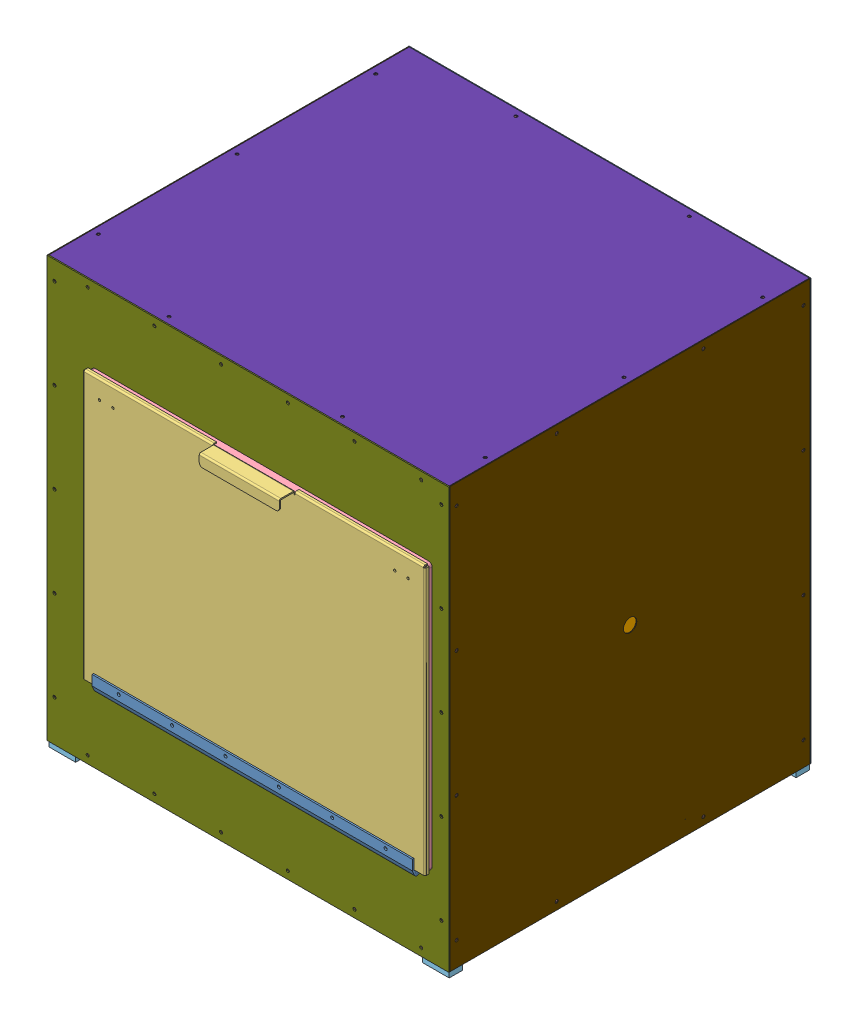
SolidWorks assembly Larva Tracker Assembly_Updated, configuration Default. Lengths in mm. (continued)
Mates (geometry in assembly coordinates): (continued)
- Distance4: distance = 1.27 mm anti-aligned: plane of Rail-2 through (-26.5232 130.7884 348.0974) normal (1 0 0); plane of Glass plate assembly-1/glass frame-1 through (-25.2532 -368.1468 246.17) normal (-1 0 0)
- Distance5: distance = 230 mm anti-aligned: plane of Camera and Lens-1/Lens Camera-1 through (6.2016 370.3134 12.6266) normal (0 -1 0); plane of Glass plate assembly-1/Glass Plate-1 through (-5.5682 140.3134 -242.565) normal (0 1 0)
- Concentric5: concentric aligned: line of BL0202 Assy-1/BL020201-1 through (6.2016 79.9884 12.6266) axis (0 1 0); cylinder of Camera and Lens-1/Lens Camera-1 through (6.2016 512.2027 12.6266) axis (0 1 0) radius 14.75
- Parallel5: parallel aligned: plane of LED Bracket-1 through (58.9721 57.0649 34.8516) normal (0 0 1); plane of Camera and Lens-1/Camera Body-1 through (-15.7984 603.427 27.1266) normal (0 0 1)
- Concentric3: concentric aligned: cylinder of T-LSR450-3/T-LSR450 Lead Screw-1 through (-65.0032 449.8358 6.0135) axis (0 0 1) radius 3.17; cylinder of Car sub assy-3/Lead Screw Nut-1 through (-65.0032 449.8358 -37.4434) axis (0 0 1) radius 3.175
- Parallel6: parallel aligned: plane of Car sub assy-3/T-LSR Top-1 through (-33.0032 436.4458 -75.8734) normal (0 -1 0); plane of T-LSR450-3/T-LSR Bearing End Plate_Thrust Bearing Version1-1 through (-97.0032 436.9282 201) normal (0 -1 0)
- Parallel7: parallel aligned: plane of T-LSR450-5/T-LSR Bearing End Plate_Thrust Bearing Version1-1 through (493.9968 394.7958 -11.3734) normal (0 -1 0); plane of Car sub assy-4/T-LSR Top-1 through (-26.0032 394.3134 -75.3734) normal (0 -1 0)
- Concentric4: concentric aligned: cylinder of T-LSR450-5/T-LSR450 Lead Screw-1 through (420.6103 407.7034 -43.3734) axis (1 0 0) radius 3.17; cylinder of Car sub assy-4/Lead Screw Nut-1 through (12.4268 407.7034 -43.3734) axis (1 0 0) radius 3.175
- Coincident52: coincident aligned: plane of Car sub assy-3/T-LSR Top-1 through (-97.0032 443.7458 -75.8734) normal (-1 0 0); plane of Zaber Bracket_Flat-3 through (-97.0032 436.4458 -75.8734) normal (-1 0 0)
- Coincident53: coincident anti-aligned: plane of Car sub assy-3/T-LSR Top-1 through (-33.0032 436.4458 -75.8734) normal (0 -1 0); plane of Zaber Bracket_Flat-3 through (-97.0032 436.4458 -10.8734) normal (0 1 0)
- Coincident54: coincident aligned: plane of Car sub assy-3/T-LSR Top-1 through (-97.0032 460.1958 -10.8734) normal (0 0 1); plane of Zaber Bracket_Flat-3 through (-97.0032 436.4458 -10.8734) normal (0 0 1)
- Coincident55: coincident anti-aligned: plane of T-LSR450-5/T-LSR450 Base-1 through (-26.0032 430.0958 -18.8734) normal (0 1 0); plane of Zaber Bracket_Flat-3 through (-97.0032 430.0958 -10.8734) normal (0 -1 0)
- Coincident56: coincident aligned: plane of T-LSR450-5/T-LSR450 Base-1 through (-26.0032 430.0958 -10.8734) normal (0 0 1); plane of Zaber Bracket_Flat-3 through (-97.0032 436.4458 -10.8734) normal (0 0 1)
- Distance6: distance = 254 mm anti-aligned: plane of Car sub assy-4/T-LSR Top-1 through (-26.0032 394.3134 -75.3734) normal (0 -1 0); plane of Glass plate assembly-1/Glass Plate-1 through (-5.5682 140.3134 -242.565) normal (0 1 0)
- Coincident60: coincident aligned: plane of T-LSR450-5/Motor Mount End Plate-1 through (-26.0032 429.5958 -11.3734) normal (1 0 0); plane of T-LSR450-2/Motor Mount End Plate-1 through (-26.0032 9.2824 -34.6134) normal (1 0 0)
- Distance9: distance = 101.6 mm anti-aligned: plane of Mini Series LED Assy-1/Mightex LED Assy-1/Mightex_Focusing Module-1 through (36.5991 241.9134 -4.9234) normal (0 -1 0); plane of Glass plate assembly-1/Glass Plate-1 through (-5.5682 140.3134 -242.565) normal (0 1 0)
- Coincident63: coincident anti-aligned: plane of Camera and Lens-1/Lens Camera-1 through (6.2016 370.3134 12.6266) normal (-0.5 0 -0.866025); plane of Mini Series LED Assy-1/Mightex LED Assy-1/Mightex_LED-1 through (36.5991 346.1734 -4.9234) normal (0.5 0 0.866025)
- Distance11: distance = 6.35 mm anti-aligned: plane of Mini Series LED Assy-1/Mightex LED Assy-1/Mightex_LED-1; cylinder of Camera and Lens-1/Lens Camera-1 through (6.2016 512.2027 12.6266) axis (0 1 0) radius 14.75
- Coincident64: coincident anti-aligned: plane of T-LSR450-5/T-LSR450 Base-1 through (-26.0032 430.0958 -18.8734) normal (0 1 0); plane of Zaber Bracket-4 through (440.7268 430.0958 -10.8734) normal (0 -1 0)
- Coincident65: coincident aligned: plane of T-LSR450-5/T-LSR450 Base-1 through (-26.0032 430.0958 -10.8734) normal (0 0 1); plane of Zaber Bracket-4 through (440.7268 436.4458 -10.8734) normal (0 0 1)
- Coincident67: coincident anti-aligned: plane of THK car-4/THK SR-15W-1 through (520.4968 448.2282 -63.1234) normal (0 -1 0); plane of Zaber Bracket-4 through (567.7268 448.2282 -75.8734) normal (0 1 0)
- Distance32: distance = 6.35 mm aligned: plane of THK car-4/THK SR-15W-1 through (508.9968 449.3282 -63.1234) normal (-1 0 0); plane of Zaber Bracket-4 through (502.6468 448.2282 -10.8734) normal (-1 0 0)
- Coincident69: coincident anti-aligned: plane of THK Rail-2 through (530.8407 459.7282 -324.9174) normal (0 -1 0); plane of THK car-4/THK SR-15W-1 through (530.8407 459.7282 -71.8734) normal (0 1 0)
- Coincident70: coincident anti-aligned: plane of THK Rail-2 through (525.9968 472.2282 -294.9174) normal (1 0 0); plane of THK car-4/THK SR-15W-1 through (525.9968 472.2282 226.6266) normal (-1 0 0)
- Coincident71: coincident aligned: plane of T-LSR450-3 through (-102.0264 419.4851 -56) normal (0 0 -1); plane of THK Rail-2
- Coincident72: coincident aligned: plane of Zaber Bracket-4 through (504.2268 430.0958 -43.3734) normal (0 0 1); plane of THK car-4/THK SR-15W-1
- Coincident75: coincident aligned: plane of Car sub assy-2/T-LSR Top-1 through (38.9968 20.8149 29.3866) normal (1 0 0); plane of Car sub assy-4/T-LSR Top-1 through (38.9968 418.0634 -11.3734) normal (1 0 0)
- Coincident76: coincident anti-aligned: plane of Car sub assy-4/T-LSR Top-1 through (-26.0032 394.3134 -75.3734) normal (0 -1 0); plane of LED Plate-1 through (-26.0032 394.3134 -11.3734) normal (0 1 0)
- Coincident77: coincident aligned: plane of Car sub assy-4/T-LSR Top-1 through (-26.0032 401.6134 -11.3734) normal (0 0 1); plane of LED Plate-1 through (-26.0032 394.3134 -11.3734) normal (0 0 1)
- Coincident78: coincident aligned: plane of Car sub assy-4/T-LSR Top-1 through (38.9968 418.0634 -11.3734) normal (1 0 0); plane of LED Plate-1 through (38.9968 394.3134 -75.3734) normal (1 0 0)
- Concentric6: concentric anti-aligned: cylinder of Camera and Lens-1/Lens Camera-1 through (6.2016 370.3134 12.6266) axis (0 -1 0) radius 12.7; cylinder of Edmund_NT63-977-1 through (6.2016 512.179 12.6266) axis (0 1 0) radius 15
- Parallel8: parallel aligned: plane of Edmund_NT63-977-1 through (16.2286 512.179 34.3766) normal (0 0 1); plane of Camera and Lens-1/Camera Body-1 through (-15.7984 603.427 27.1266) normal (0 0 1)
- Coincident80: coincident anti-aligned: plane of Camera and Lens-1/Camera Body-1 through (-15.7984 603.427 27.1266) normal (0 0 1); plane of Camera Bracket_3-1 through (-15.7984 662.427 27.1266) normal (0 0 -1)
- Coincident81: coincident aligned: plane of Camera Bracket_3-1 through (-15.7984 662.427 27.1266) normal (0 1 0); plane of Camera and Lens-1/Camera Body-1 through (28.2016 662.427 27.1266) normal (0 1 0)
- Coincident82: coincident aligned: plane of Camera and Lens-1/Camera Body-1 through (-15.7984 603.427 27.1266) normal (-1 0 0); plane of Camera Bracket_3-1 through (-15.7984 499.479 27.1266) normal (-1 0 0)
- Distance15: distance = 63.5 mm anti-aligned: plane of Edmund_NT63-977-1 through (6.2016 524.879 12.6266) normal (0 1 0); plane of Camera and Lens-1/Lens Camera-1 through (18.9016 588.379 12.6266) normal (0 -1 0)
- Coincident90: coincident anti-aligned: plane of LED Plate-1 through (19.9664 386.0584 -75.3734) normal (0 1 0); plane of Camera Bracket-1 through (-18.3384 386.0584 40.6836) normal (0 -1 0)
- Coincident92: coincident anti-aligned: plane of Camera Bracket-1 through (21.0606 478.397 55.9236) normal (0 0 -1); plane of Thor Lab MS1 stage 6132-E0W-1 through (-8.6574 448.679 55.9236) normal (0 0 1)
- Coincident100: coincident anti-aligned: plane of Rexroth-8 981 021 399_-1 through (-25.1987 -34.9496 297.3) normal (0 0 1); plane of Rexroth-8 981 021 399_-7 through (-174.9591 -28.9999 297.3) normal (0 0 -1)
- Distance18: distance = 12.7 mm aligned: plane of Rexroth-8 981 021 399_-2 through (-174.9591 -28.9999 -337.7) normal (0 0 -1); plane of T-LSR450-3/Motor Mount End Plate-1 through (-97.0032 471.7282 -325) normal (0 0 -1)
- Coincident104: coincident aligned: plane of Rexroth-8 981 021 399_-2 through (-174.9591 -44.4491 -287.1026) normal (-1 0 0); plane of Rexroth-8 981 021 399_-4 through (-174.9591 -44.4491 297.2974) normal (-1 0 0)
- Coincident105: coincident anti-aligned: plane of Rexroth-8 981 021 399_-2 through (-174.9591 -34.9496 -286.9026) normal (0 0 1); plane of Rexroth-8 981 021 399_-4 through (-174.7591 -34.9496 -286.9026) normal (0 0 -1)
- Coincident106: coincident anti-aligned: plane of Rexroth-8 981 021 399_-6 through (-167.0095 -27 297.5) normal (0 -1 0); plane of Rexroth-8 981 021 399_-4 through (-167.0095 -27 297.2974) normal (0 1 0)
- Distance19: distance = 12.7 mm aligned: plane of Rexroth-8 981 021 399_-2 through (581.6968 -44.4491 -287.1026) normal (1 0 0); plane of Zaber Bracket-4 through (568.9968 426.9081 -318) normal (1 0 0)
- Coincident110: coincident anti-aligned: plane of T-LSR450-3/T-LSR450 Base-1 through (-60.5032 472.2282 -319) normal (0 1 0); plane of Rexroth-8 981 021 399_-8 through (-72.9528 472.2282 297.3) normal (0 -1 0)
- Coincident111: coincident aligned: plane of Rexroth-8 981 021 399_-8; plane of Car sub assy-3/Lead Screw Nut-1
- Coincident119: coincident aligned: plane of Rexroth-8 981 021 399_-6 through (-167.0095 -27 348.0974) normal (0 0 1); plane of Rexroth-8 981 021 399_-7 through (-174.9591 -50.3988 348.0974) normal (0 0 1)
- Coincident123: coincident aligned: plane of Rexroth-8 981 021 399_-6 through (-174.9591 -27 330.6483) normal (-1 0 0); plane of Rexroth-8 981 021 399_-7 through (-174.9591 -44.4491 347.8974) normal (-1 0 0)
- Coincident130: coincident anti-aligned: plane of Rail-1 through (465.3868 121.2634 -337.7026) normal (0 -1 0); plane of Rexroth-8 981 021 399_-13 through (561.6396 121.2634 314.7491) normal (0 1 0)
- Coincident131: coincident aligned: plane of Rexroth-8 981 021 399_-7 through (-174.9591 -34.9496 348.0974) normal (0 0 1); plane of Rexroth-8 981 021 399_-13 through (561.6396 119.2635 348.0974) normal (0 0 1)
- Coincident132: coincident anti-aligned: plane of Rexroth-8 981 021 399_-6 through (-149.5604 -27 314.7491) normal (1 0 0); plane of Rexroth-8 981 021 399_-13 through (-149.5604 113.3138 347.8974) normal (-1 0 0)
- Coincident133: coincident anti-aligned: plane of Rexroth-8 981 021 399_-6 through (-172.9592 -27 297.3) normal (0 0 -1); plane of Rexroth-8 981 021 399_-8 through (-39.8045 480.1778 297.3) normal (0 0 1)
- Coincident134: coincident aligned: plane of Rexroth-8 981 021 399_-8 through (-57.0536 497.6269 297.3) normal (0 1 0); plane of Rexroth-8 981 021 399_-15 through (-149.5604 497.6269 330.6483) normal (0 1 0)
- Coincident136: coincident anti-aligned: plane of Rexroth-8 981 021 399_-6 through (-149.5604 -27 314.7491) normal (1 0 0); plane of Rexroth-8 981 021 399_-15 through (-149.5604 489.6773 297.5) normal (-1 0 0)
- Coincident137: coincident anti-aligned: plane of Back Sheet -1 through (588.6271 -53.9862 -337.7) normal (0 0 1); plane of Side Sheet -2 through (587.0396 746.1125 -337.7) normal (0 0 -1)
- Coincident138: coincident anti-aligned: plane of Front Sheet -1 through (-176.5466 -53.9862 348.0974) normal (0 0 -1); plane of Rexroth-8 981 021 399_-6 through (-167.0095 -27 348.0974) normal (0 0 1)
- Coincident144: coincident anti-aligned: plane of Rexroth-8 981 021 399_-20 through (569.5892 744.525 297.2974) normal (0 1 0); plane of Top Sheet -1 through (-174.9604 744.525 -337.7032) normal (0 -1 0)
- Coincident147: coincident anti-aligned: plane of Rexroth-8 981 021 399_-11 through (-174.9591 -27 -304.3517) normal (-1 0 0); plane of Side Sheet -1 through (-174.9591 -53.9862 -337.7) normal (1 0 0)
- Coincident149: coincident aligned: plane of Side Sheet -1 through (-176.5466 -53.9862 -337.7) normal (0 -1 0); plane of Bottom Sheet -1 through (587.0396 -53.9862 -337.7) normal (0 -1 0)
- Coincident150: coincident aligned: plane of Rexroth-8 981 021 399_-11 through (-157.51 -27 -337.7) normal (0 0 -1); plane of Side Sheet -1 through (-176.5466 746.1125 -337.7) normal (0 0 -1)
- Coincident151: coincident anti-aligned: plane of Rexroth-8 981 021 399_-3 through (487.3439 -52.3987 297.3) normal (0 -1 0); plane of Bottom Sheet -1 through (587.0396 -52.3987 -337.7) normal (0 1 0)
- Coincident152: coincident aligned: plane of Rexroth-8 981 021 399_-12 through (587.0396 -27 -320.2509) normal (1 0 0); plane of Bottom Sheet -1 through (587.0396 -53.9862 348.1) normal (1 0 0)
- Coincident153: coincident aligned: plane of Rexroth-8 981 021 399_-12 through (579.09 -27 -337.7) normal (0 0 -1); plane of Bottom Sheet -1 through (587.0396 -53.9862 -337.7) normal (0 0 -1)
- Coincident172: coincident anti-aligned: plane of Front Sheet -1 through (-176.5466 -53.9862 350.3834) normal (0 0 1); plane of 1581A167_Hinge-1 through (-72.044 116.4253 350.3834) normal (0 0 -1)
- Coincident174: coincident anti-aligned: plane of Glass plate assembly-1/Glass Plate-1 through (232.1318 130.7757 -4.865) normal (1 0 0); plane of 1581A167_Hinge-1 through (232.1318 78.1814 351.9074) normal (-1 0 0)
- Coincident176: coincident anti-aligned: plane of Camera Bracket_3-1 through (-15.7984 531.4652 40.6836) normal (0 0 1); plane of Thor Lab MS1 stage 6132-E0W-1 through (-0.6833 478.397 40.6836) normal (0 0 -1)
- Coincident177: coincident aligned: plane of Camera Bracket_3-1; plane of Thor Lab MS1 stage 6132-E0W-1
- Coincident178: coincident aligned: plane of Camera Bracket_3-1 through (-15.7984 448.679 40.6836) normal (0 -1 0); plane of Thor Lab MS1 stage 6132-E0W-1 through (21.0606 448.679 42.0806) normal (0 -1 0)
- Distance25: distance = 2.54 mm anti-aligned: plane of Camera Bracket-1 through (-18.3384 392.4084 8.9336) normal (1 0 0); plane of Camera Bracket_3-1 through (-15.7984 499.479 27.1266) normal (-1 0 0)
- Coincident185: coincident aligned: plane of Top Sheet -1 through (-174.9604 744.525 5.1974) normal (0 0 1); plane of Rexroth-8 981 021 399_-19 through (-149.5604 731.8257 5.1974) normal (0 0 1)
- Coincident186: coincident aligned: plane of Top Sheet -1; plane of Rexroth-8 981 021 399_-17 through (206.0396 731.8383 322.6987) normal (-1 0 0)
- Distance31: distance = 5.9026 mm aligned: plane of THK car-3/THK SR-15W-1 through (499.5942 -4.1 -22.3634) normal (1 0 0); plane of Bottom Slider Bracket-1 through (505.4968 8.7824 -35.1134) normal (1 0 0)
- Coincident193: coincident anti-aligned: plane of THK Rail-2 through (525.9968 472.2282 -294.9174) normal (1 0 0); plane of Rexroth-8 981 021 399_-9
- Coincident198: coincident aligned: plane of Rail-1 through (506.6618 121.2634 5.1974) normal (0 0 1); plane of Rexroth-8 981 021 399_-4 through (-149.5604 -39.6993 5.1974) normal (0 0 1)
- Coincident219: coincident anti-aligned: plane of T-LSR450-2/Motor Mount End Plate-1 through (-26.0032 9.2824 -164.54) normal (1 0 0); plane of Car sub assy-2/T-LSR Top-1 through (-26.0032 20.8149 -100.54) normal (-1 0 0)
- Coincident175: coincident anti-aligned: plane of Door Assembly-1/Door-1 through (-91.0197 605.5023 365.8774) normal (0 0 1); plane of 1581A167_Hinge-1 through (-59.344 97.2483 365.8774) normal (0 0 -1)
- Distance22: distance = 25.146 mm anti-aligned: plane of Door Assembly-1/Door-1 through (-91.0197 97.5023 365.8774) normal (0 -1 0); plane of Front Sheet -1 through (-59.2697 122.6483 348.0974) normal (0 1 0)
- Distance23: distance = 25.4 mm aligned: plane of Door Assembly-1/Door-1 through (-91.0197 605.5023 363.5914) normal (1 0 0); plane of Front Sheet -1 through (-65.6197 566.6086 348.0974) normal (1 0 0)
- Coincident1: coincident aligned: plane of T-LSR450-6 through (0 25.7431 -379.7755) normal (1 0 0); plane of assembly
- Distance33: distance = 15.24 mm anti-aligned: plane of T-LSR450-6 through (37.02 25.7431 -15.24) normal (0 0 -1); plane of assembly
- Coincident25: coincident aligned: plane of T-LSR450-6 through (37.02 25.7431 -15.24) normal (0 0 -1); plane of THK Rail-1 through (482.5942 -27 -15.24) normal (0 0 -1)
- Coincident97: coincident aligned: plane of T-LSR450-6 through (0 25.7431 -379.7755) normal (1 0 0); plane of Rexroth-8 981 021 399_-1
- Coincident3: coincident aligned: plane of assembly; plane of T-LSR450-6/T-LSR450 Base-1 through (24.742 0 -278.24) normal (0 1 0)
- Distance7: distance = 65 mm aligned: plane of T-LSR450-3/T-LSR450 Base-1 through (-97.5032 451.2282 -319) normal (-1 0 0); plane of T-LSR450-6/T-LSR450 Base-1 through (-32.5032 -6 241.76) normal (-1 0 0)
- Coincident93: coincident anti-aligned: plane of T-LSR450-6/T-LSR450 Base-1 through (24.4968 -27 -278.24) normal (0 -1 0); plane of Rexroth-8 981 021 399_-1 through (7.9496 -27 297.3) normal (0 1 0)
- Coincident164: coincident anti-aligned: plane of T-LSR450-6/T-LSR450 Base-1 through (-32.5032 -27 -278.24) normal (0 -1 0); plane of Rexroth-8 981 021 399_-7 through (-174.9591 -27 330.6483) normal (0 1 0)
- Coincident5: coincident anti-aligned: plane of Car sub assy-5/T-LSR Top-1 through (-32.0032 8.7824 -35.1134) normal (0 1 0); plane of T-LSR450-2/T-LSR450 Base-1 through (-26.0032 8.7824 1.8866) normal (0 -1 0)
- Coincident6: coincident aligned: plane of T-LSR450-2/Motor Mount End Plate-1 through (-32.0032 9.2824 -34.6134) normal (-1 0 0); plane of Car sub assy-5/T-LSR Top-1 through (-32.0032 1.4824 29.8866) normal (-1 0 0)
- Coincident7: coincident aligned: plane of Car sub assy-5/T-LSR Top-1 through (31.9968 -14.9676 -35.1134) normal (0 0 -1); plane of T-LSR450-2/T-LSR450 Base-1 through (-26.0032 8.7824 -35.1134) normal (0 0 -1)
- Distance13: distance = 40.76 mm aligned: plane of Car sub assy-3/T-LSR Top-1 through (-97.0032 460.1958 -10.8734) normal (0 0 1); plane of Car sub assy-5/T-LSR Top-1 through (31.9968 -14.9676 29.8866) normal (0 0 1)
- Concentric1: concentric anti-aligned: circle of T-LSR450-6/T-LSR450 Lead Screw-1; cylinder of Car sub assy-5/Lead Screw Nut-1 through (-0.0032 -4.6076 3.3166) axis (0 0 1) radius 3.175
- Parallel1: parallel aligned: plane of T-LSR450-6/T-LSR450 Base-1 through (-32.5032 0 -278.24) normal (0 1 0); plane of Car sub assy-5/T-LSR Top-1 through (-32.0032 8.7824 -35.1134) normal (0 1 0)
- Coincident34: coincident anti-aligned: plane of T-LSR450-6/Motor Mount End Plate-1 through (31.9968 -26.5 -278.24) normal (0 0 1); plane of Car sub assy-5/T-LSR Top-1 through (31.9968 -14.9676 -278.24) normal (0 0 -1)
- Coincident102: coincident anti-aligned: plane of T-LSR450-6/T-LSR Bearing End Plate_Thrust Bearing Version1-1 through (-32.0032 -26.5 241.76) normal (0 0 -1); plane of Car sub assy-5/T-LSR Top-1 through (31.9968 -14.9676 241.76) normal (0 0 1)
- Coincident222: coincident anti-aligned: plane of Rexroth-8 981 021 399_-13; plane of Rexroth-8 981 021 399_-15
- Concentric7: concentric aligned: circle of 1581A167_Hinge-1; circle of Front Sheet -1
- Parallel9: parallel aligned: plane of Front Sheet -1 through (-59.2697 122.6483 348.0974) normal (0 1 0); plane of 1581A167_Hinge-1 through (-59.344 116.4253 365.8774) normal (0 1 0)
- Coincident223: coincident aligned: plane of Front Sheet -1 through (-176.5466 746.1125 350.3834) normal (0 1 0); plane of Top Sheet -1 through (-174.9604 746.1125 -337.7032) normal (0 1 0)
- Coincident224: coincident aligned: plane of Front Sheet -1 through (588.6271 746.1125 350.3834) normal (1 0 0); plane of Side Sheet -2 through (588.6271 -53.9862 -337.7) normal (1 0 0)
- Coincident229: coincident aligned: plane of Back Sheet -1 through (588.6271 746.1125 -339.2875) normal (0 1 0); plane of Top Sheet -1 through (-174.9604 746.1125 -337.7032) normal (0 1 0)
- Coincident230: coincident aligned: plane of Back Sheet -1 through (588.6271 746.1125 -339.2875) normal (1 0 0); plane of Side Sheet -2 through (588.6271 -53.9862 -337.7) normal (1 0 0)
- Coincident233: coincident anti-aligned: plane of ? through (6.4968 57.0522 -106.9966) normal (1 0 0)
- Distance38: distance = 15.24 mm aligned: plane of Car sub assy-2/T-LSR Top-1 through (38.9968 21.0649 -2.6134) normal (0 0 1); plane of BL0202 Assy-1/BL020201-1 through (6.2016 57.0649 12.6266) normal (0 0 1)
- Coincident234: coincident anti-aligned: plane of Rexroth-8 981 021 399_-7 through (-174.9591 -52.3987 340.1478) normal (0 -1 0); plane of 8020_2128-1 through (536.2409 -52.3987 348.0974) normal (0 1 0)
- Coincident235: coincident aligned: plane of Rexroth-8 981 021 399_-7 through (587.0409 -44.4491 347.8974) normal (1 0 0); plane of 8020_2128-1 through (587.0409 -65.0987 348.0974) normal (1 0 0)
- Coincident236: coincident: line of Rexroth-8 981 021 399_-7 through (587.0409 -50.3988 348.0974) axis (0 1 0); plane of 8020_2128-1 through (587.0409 -65.0987 348.0974) normal (0 0 1)
- Coincident237: coincident anti-aligned: plane of Front Sheet -1 through (-176.5466 -53.9862 350.3834) normal (0 0 1); plane of Spacer Block-1 through (-65.6197 580.1023 350.3834) normal (0 0 -1)
- Concentric13: concentric anti-aligned: cylinder of Front Sheet -1 through (-60.8572 572.5617 350.3834) axis (0 0 1) radius 2.25; cylinder of Spacer Block-1 through (-60.8572 572.5617 350.3834) axis (0 0 -1) radius 2.25
- Concentric14: concentric anti-aligned: cylinder of Front Sheet -1 through (-35.4572 572.5617 350.3834) axis (0 0 1) radius 2.25; cylinder of Spacer Block-1 through (-35.4572 572.5617 350.3834) axis (0 0 -1) radius 2.25
- Coincident240: coincident anti-aligned: plane of 1745A12_bracket-4 through (-30.6947 565.0211 361.153) normal (0 0 -1); plane of Spacer Block-1 through (-65.6197 580.1023 361.153) normal (0 0 1)
- Concentric15: concentric anti-aligned: cylinder of 1745A12_magnet-7 through (-35.4572 572.5617 361.607) axis (0 0 1) radius 2.1; cylinder of Spacer Block-1 through (-35.4572 572.5617 350.3834) axis (0 0 -1) radius 2.25
- Concentric16: concentric anti-aligned: cylinder of 1745A12_magnet-7 through (-60.8572 572.5617 361.607) axis (0 0 1) radius 2.1; cylinder of Spacer Block-1 through (-60.8572 572.5617 350.3834) axis (0 0 -1) radius 2.25
- Coincident241: coincident anti-aligned: plane of 1745A12_magnet-7 through (-30.6947 566.6086 363.5914) normal (0 0 1); plane of Door Assembly-1/Door-1 through (-91.0197 605.5023 363.5914) normal (0 0 -1)
- Coincident243: coincident anti-aligned: plane of T-LSR450-5/Motor Mount End Plate-1 through (-26.0032 429.5831 -300.6654) normal (1 0 0); plane of Car sub assy-4/T-LSR Top-1 through (-26.0032 418.0507 -300.6654) normal (-1 0 0)
- Coincident245: coincident anti-aligned: plane of Rexroth-8 981 021 399_-10 through (579.09 -27 297.3) normal (0 0 -1); plane of Rexroth-8 981 021 399_-21 through (569.5905 -52.1987 297.3) normal (0 0 1)
- Coincident246: coincident aligned: plane of Rexroth-8 981 021 399_-21 through (587.0396 -34.9496 297.3) normal (1 0 0); plane of Rexroth-8 981 021 399_-10 through (587.0396 -27 314.7491) normal (1 0 0)
- Coincident247: coincident anti-aligned: plane of Bottom Sheet -1 through (587.0396 -52.3987 -337.7) normal (0 1 0); plane of Rexroth-8 981 021 399_-21 through (579.09 -52.3987 297.3) normal (0 -1 0)
- Coincident248: coincident anti-aligned: plane of LED Bracket-1 through (6.2016 44.5649 12.6266) normal (-1 0 0); plane of BL0202 Assy-1/BL020201-1 through (6.2016 57.0649 48.7454) normal (1 0 0)
- Coincident249: coincident anti-aligned: plane of LED Bracket-1 through (6.2016 57.0649 -9.5984) normal (0 1 0); plane of BL0202 Assy-1/BL020201-1 through (-29.5362 57.0649 48.7454) normal (0 -1 0)
- PLANE1: unknown = 38.5 mm: plane of T-LSR450-2/Motor Mount End Plate-1 through (-32.0032 9.2824 -34.6134) normal (-1 0 0)
- PLANE2: unknown: plane of T-LSR450-6/Motor Mount End Plate-1 through (31.9968 -26.5 -278.24) normal (0 0 1); unknown of Edmund_NT63-977-1
- LocalLPattern2: unknown: line of T-LSR450-6/T-LSR450 Base-1 through (-32.5032 -21 241.76) axis (0 0 -1)
- LocalLPattern3: unknown: line of T-LSR450-6/T-LSR450 Base-1 through (-32.5032 -21 241.76) axis (0 0 -1)
- LocalLPattern4: unknown: line of T-LSR450-5/T-LSR450 Base-1 through (493.9968 403.0958 -10.8734) axis (-1 0 0)
- LocalLPattern5: unknown: line of T-LSR450-6/T-LSR450 Base-1 through (-32.5032 -21 241.76) axis (0 0 -1); line of T-LSR450-2/T-LSR450 Base-1 through (-26.0032 8.7824 29.8866) axis (1 0 0)
- LocalLPattern6: unknown: line of T-LSR450-6/T-LSR450 Base-1 through (-32.5032 -6 -278.24) axis (0 0 1)
- LocalLPattern7: unknown: line of T-LSR450-3/T-LSR450 Base-1 through (-97.5032 445.2282 201) axis (0 0 -1); line of T-LSR450-5/Motor Mount End Plate-1 through (-26.0032 387.5958 -11.3734) axis (0 1 0)
- LocalLPattern8: unknown: line of T-LSR450-6/Motor Mount End Plate-1 through (-32.0032 -26.5 -278.24) axis (0 1 0)
- LocalLPattern9: unknown: line of Rexroth-8 981 021 399_-19 through (-174.9591 742.5251 297.2974) axis (0 0 -1); line of T-LSR450-5/T-LSR450 Base-1 through (493.9968 403.0958 -10.8734) axis (-1 0 0)
- LocalLPattern10: unknown: line of T-LSR450-5/T-LSR450 Base-1 through (493.9968 403.0958 -75.8734) axis (-1 0 0); unknown of Rexroth-8 981 021 399_-3; unknown of T-LSR450-2/T-LSR450 Base-1; unknown of T-LSR450-2/T-LSR450 Base-1; unknown of T-LSR450-2/T-LSR450 Base-1; unknown of T-LSR450-2/T-LSR450 Base-1; unknown of T-LSR450-2/T-LSR450 Base-1; unknown of T-LSR450-2/T-LSR450 Base-1; unknown of T-LSR450-2/T-LSR450 Base-1; unknown of T-LSR450-2/T-LSR450 Base-1; unknown of THK car-3/THK SR-15W-1; unknown of THK car-3/THK SR-15W-1; unknown of THK car-3/THK SR-15W-1; unknown of THK car-3/THK SR-15W-1; unknown of THK car-3/THK SR-15W-1; unknown of THK car-3/THK SR-15W-1; unknown of THK car-3/THK SR-15W-1; unknown of THK car-3/THK SR-15W-1; unknown of THK car-3/THK SR-15W-1; unknown of THK car-3/THK SR-15W-1; unknown of THK car-3/THK SR-15W-1; unknown of THK car-4/THK SR-15W-1; unknown of THK car-4/THK SR-15W-1; unknown of THK car-4/THK SR-15W-1; unknown of THK car-4/THK SR-15W-1; unknown of THK car-4/THK SR-15W-1; unknown of THK car-4/THK SR-15W-1; unknown of THK car-4/THK SR-15W-1; unknown of THK car-4/THK SR-15W-1; unknown of T-LSR450-5/T-LSR450 Base-1; unknown of T-LSR450-5/T-LSR450 Base-1; unknown of T-LSR450-5/T-LSR450 Base-1; unknown of T-LSR450-5/T-LSR450 Base-1; unknown of T-LSR450-5/T-LSR450 Base-1; unknown of T-LSR450-5/T-LSR450 Base-1; unknown of T-LSR450-5/T-LSR450 Base-1; unknown of T-LSR450-5/T-LSR450 Base-1; unknown of Car sub assy-4/T-LSR Top-1; unknown of Car sub assy-4/T-LSR Top-1; unknown of Car sub assy-4/T-LSR Top-1; unknown of Car sub assy-4/T-LSR Top-1; unknown of Car sub assy-4/T-LSR Top-1; unknown of Car sub assy-4/T-LSR Top-1; unknown of Car sub assy-4/T-LSR Top-1; unknown of Car sub assy-4/T-LSR Top-1; unknown of Camera and Lens-1/Camera Body-1; unknown of Camera and Lens-1/Camera Body-1; unknown of Camera and Lens-1/Camera Body-1; unknown of Camera and Lens-1/Camera Body-1; unknown of T-LSR450-5/T-LSR450 Base-1; unknown of T-LSR450-5/T-LSR450 Base-1; unknown of T-LSR450-5/T-LSR450 Base-1; unknown of T-LSR450-5/T-LSR450 Base-1; unknown of T-LSR450-5/T-LSR450 Base-1; unknown of T-LSR450-5/T-LSR450 Base-1; unknown of T-LSR450-5/T-LSR450 Base-1; unknown of T-LSR450-5/T-LSR450 Base-1; unknown of Car sub assy-3/T-LSR Top-1; unknown of Car sub assy-3/T-LSR Top-1; unknown of Car sub assy-3/T-LSR Top-1; unknown of Car sub assy-3/T-LSR Top-1; unknown of Car sub assy-3/T-LSR Top-1; unknown of Car sub assy-3/T-LSR Top-1; unknown of Car sub assy-3/T-LSR Top-1; unknown of Car sub assy-3/T-LSR Top-1; unknown of Mini Series LED Assy-3/8587-E0W-1; unknown of Mini Series LED Assy-3/8587-E0W-1; unknown of Mini Series LED Assy-1/8587-E0W-1; unknown of Mini Series LED Assy-1/8587-E0W-1; unknown of Mini Series LED Assy-2/8587-E0W-1; unknown of Mini Series LED Assy-2/8587-E0W-1; unknown of Mini Series LED Assy-3/8587-E0W-1; unknown of Mini Series LED Assy-3/8587-E0W-1; unknown of Mini Series LED Assy-1/8587-E0W-1; unknown of Mini Series LED Assy-1/8587-E0W-1; unknown of Mini Series LED Assy-2/8587-E0W-1; unknown of Mini Series LED Assy-2/8587-E0W-1; unknown of Mini Series LED Assy-3/8587-E0W-1; unknown of Mini Series LED Assy-3/8587-E0W-1; unknown of Mini Series LED Assy-1/8587-E0W-1; unknown of Mini Series LED Assy-1/8587-E0W-1; unknown of Mini Series LED Assy-2/8587-E0W-1; unknown of Mini Series LED Assy-2/8587-E0W-1; unknown of Mini Series LED Assy-3/8587-E0W-1; unknown of Mini Series LED Assy-3/8587-E0W-1; unknown of Mini Series LED Assy-1/8587-E0W-1; unknown of Mini Series LED Assy-1/8587-E0W-1; unknown of Mini Series LED Assy-2/8587-E0W-1; unknown of Mini Series LED Assy-2/8587-E0W-1; unknown of Thor Lab MS1 stage 6132-E0W-1; unknown of Thor Lab MS1 stage 6132-E0W-1; unknown of Thor Lab MS1 stage 6132-E0W-1; unknown of Thor Lab MS1 stage 6132-E0W-1; unknown of Thor Lab MS1 stage 6132-E0W-1; unknown of Thor Lab MS1 stage 6132-E0W-1; unknown of Thor Lab MS1 stage 6132-E0W-1; unknown of Thor Lab MS1 stage 6132-E0W-1; unknown of Thor Lab MS1 stage 6132-E0W-1; unknown of Thor Lab MS1 stage 6132-E0W-1; unknown of Thor Lab MS1 stage 6132-E0W-1; unknown of Thor Lab MS1 stage 6132-E0W-1; unknown of Camera Bracket-1; unknown of Camera Bracket-1; unknown of Camera Bracket-1; unknown of Camera Bracket-1; unknown of T-LSR450-6/T-NM17 Housing-1; unknown of T-LSR450-6/T-NM17 Housing-1; unknown of T-LSR450-6/T-NM17 Housing-1; unknown of T-LSR450-6/T-NM17 Housing-1; unknown of T-LSR450-6/T-NM17 Housing-1; unknown of T-LSR450-6/T-NM17 Housing-1; unknown of T-LSR450-6/T-NM17 Housing-1; unknown of T-LSR450-6/T-NM17 Housing-1; unknown of T-LSR450-3/T-NM17 Housing-1; unknown of T-LSR450-3/T-NM17 Housing-1; unknown of T-LSR450-3/T-NM17 Housing-1; unknown of T-LSR450-3/T-NM17 Housing-1; unknown of T-LSR450-3/T-NM17 Housing-1; unknown of T-LSR450-3/T-NM17 Housing-1; unknown of T-LSR450-3/NM17-H-1; unknown of T-LSR450-3/T-NM17 Housing-1; unknown of T-LSR450-3/T-NM17 Housing-1; unknown of T-LSR450-3/T-NM17 Housing-1; unknown of T-LSR450-3/T-NM17 Housing-1; unknown of T-LSR450-3/T-NM17 Housing-1; unknown of T-LSR450-3/T-NM17 Housing-1; unknown of T-LSR450-3/T-NM17 Housing-1; unknown of T-LSR450-3/T-NM17 Housing-1; unknown of T-LSR450-3/T-NM17 Housing-1; unknown of T-LSR450-3/T-NM17 Housing-1; unknown of T-LSR450-6/T-NM17 Housing-1; unknown of T-LSR450-6/T-NM17 Housing-1; unknown of T-LSR450-6/T-NM17 Housing-1; unknown of T-LSR450-6/T-NM17 Housing-1; unknown of T-LSR450-6/T-NM17 Housing-1; unknown of T-LSR450-6/T-NM17 Housing-1; unknown of T-LSR450-6/T-NM17 Housing-1; unknown of T-LSR450-6/T-NM17 Housing-1; unknown of T-LSR450-5; unknown of T-LSR450-5; unknown of Rexroth-8 981 021 399_-3
- LocalLPattern11: unknown: line of Rexroth-8 981 021 399_-3 through (518.6923 -52.3987 297.3) axis (0 0 -1); line of Rexroth-8 981 021 399_-7 through (-174.9591 -52.3987 340.1478) axis (1 0 0)
- LocalLPattern12: unknown: line of Front Sheet -1 through (496.3553 579.8483 350.3834) axis (-1 0 0)
- LocalLPattern13: unknown: line of Door Assembly-1/Door-1 through (-90.3126 605.5023 358.5114) axis (1 0 0); unknown of Camera and Lens-1; unknown of Camera and Lens-1
